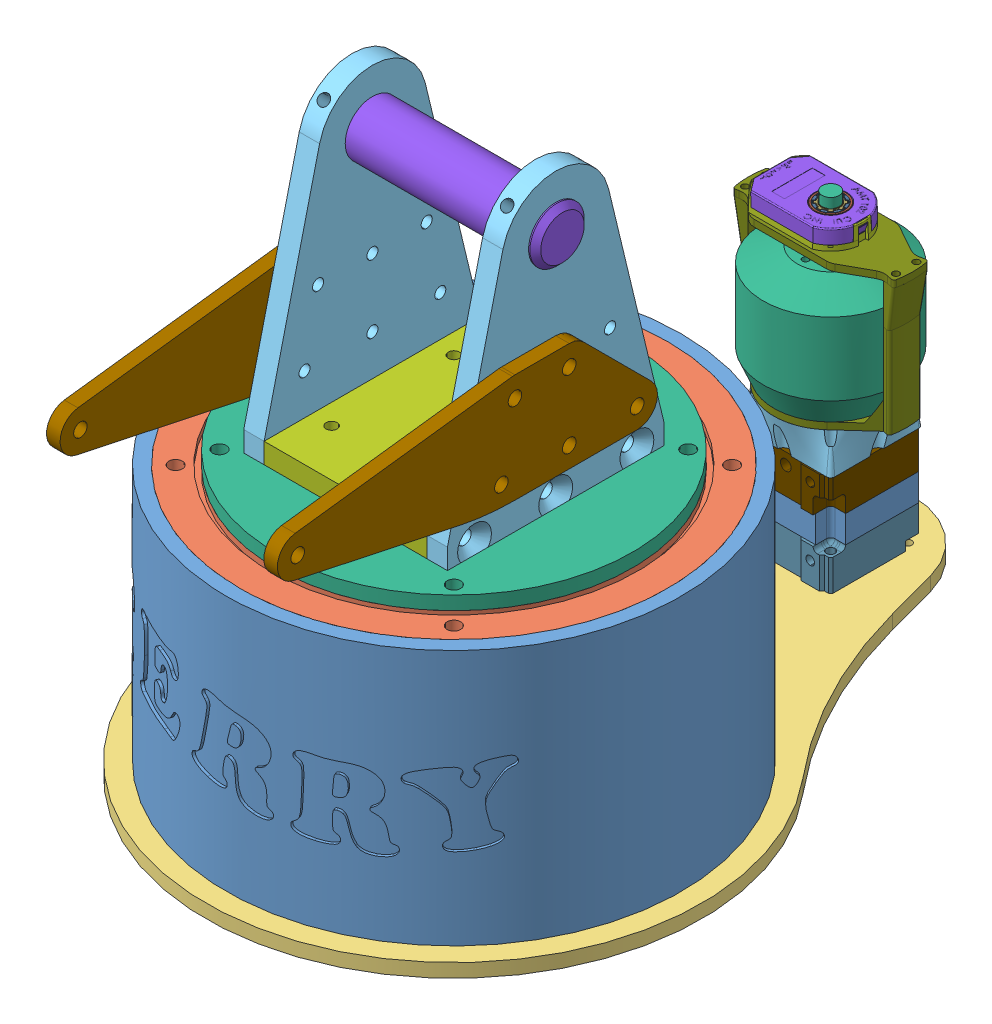
SolidWorks assembly Base, configuration Default. Lengths in mm.
Overall size (231.75 300.27 350.82).
75 component instances, 49 part files, 14 mates.
Components (placement in the parent):
- BotTurretHousing^Base-1: BotTurretHousing^Base [Default] at origin size (212.7 119.6 212.71) (virtual)
- 8in-1: 8in [Default] at (0 55.3 0) size (200 9 200)
- 8in-2: 8in [Default] at (0 -55.3 0) x (1 0 0) z (0 0 -1) size (200 9 200)
- BasePlate^Base-1: BasePlate^Base [Default] at origin size (231.75 6.35 330.18) (virtual)
- BotTurretPlate^Base-1: BotTurretPlate^Base [Default] at origin size (166.96 6.35 166.96) (virtual)
- SideTurretPlate^Base-1: SideTurretPlate^Base [Default] at origin size (9.52 262.48 101.23) (virtual)
- SideTurretPlate^Base-3: SideTurretPlate^Base [Default] x (-1 0 0) z (0 0 -1) size (9.52 262.48 101.23) (virtual)
- TopTurretPlate^Base-1: TopTurretPlate^Base [Default] at origin size (166.96 6.35 166.96) (virtual)
- TopBrace^Base-1: TopBrace^Base [Default] at origin size (76.2 9.53 101.23) (virtual)
- 6061K602_HARDENED PRECISION STEEL SHAFT-1: 6061K602_HARDENED PRECISION STEEL SHAFT [6061K602] at (0 177.275 0) size (101.6 25.4 25.4)
- PivotPlate^Base-1: PivotPlate^Base [Default] at origin size (6.35 50.8 177.8) (virtual)
- PivotPlate^Base-2: PivotPlate^Base [Default] at (101.6 0 0) size (6.35 50.8 177.8) (virtual)
- Keda9to1-1: Keda9to1 [Default] at (0 -43.175 -153.975) x (0 -1 0) z (1 0 0) size (176.96 63 76.93)
  - VersaPlanetary_v2_Single_Stage_10_1_with_BAG.STEP-1: VersaPlanetary_v2_Single_Stage_10_1_with_BAG.STEP [Default] at origin size (163.4 63.52 63.52)
    - 217-2820 Rev1_Public.STEP-1: 217-2820 Rev1_Public.STEP [Default] at (-4.6546 22.225 0) x (0 -0.456494 0.889726) z (-1 0 0) size (39.22 38.88 17.4)
      - 217-2625-100.STEP-1: 217-2625-100.STEP [Default] at origin size (39.22 38.88 12.7)
        - 217-2625-008 Rev1.STEP-1: 217-2625-008 Rev1.STEP [Default] at origin size (34.7 34.7 4.7)
        - 217-2625-010 Rev1.STEP-1: 217-2625-010 Rev1.STEP [Default] at (0 10.193 3.65) x (0.999813 0.019336 0) z (0 0 1) size (4 4 12)
        - 217-2625-010 Rev1.STEP-2: 217-2625-010 Rev1.STEP [Default] at (8.691 -5.3258 3.65) size (4 4 12)
        - 217-2625-010 Rev1.STEP-3: 217-2625-010 Rev1.STEP [Default] at (-8.691 -5.3258 3.65) size (4 4 12)
        - 217-2625-005 Rev1_Planet_Revolving_Follower01.STEP-1: 217-2625-005 Rev1_Planet_Revolving_Follower01.STEP [Default] at (8.691 -5.3258 6.35) x (0.932816 0.360354 0) z (0 0 1) size (16.89 16.89 8)
        - 217-2625-005 Rev1_Planet_Revolving_Follower01.STEP-2: 217-2625-005 Rev1_Planet_Revolving_Follower01.STEP [Default] at (-8.691 -5.3258 6.35) x (-0.932788 -0.360426 0) z (0 0 1) size (16.89 16.89 8)
        - 217-2625-005 Rev1_Planet_Revolving_Follower01.STEP-3: 217-2625-005 Rev1_Planet_Revolving_Follower01.STEP [Default] at (0 10.193 6.35) x (0.893583 0.448898 0) z (0 0 1) size (16.89 16.89 8)
      - 217-2625-007 Rev1_Public.STEP-1: 217-2625-007 Rev1_Public.STEP [Default] at (0 0 6.7) x (0.992772 0.120019 0) z (0 0 1) size (15.27 15.27 12.7)
    - 217-2625-026 Rev1.STEP-1: 217-2625-026 Rev1.STEP [Default] at (-6.5 22.225 0) x (0 -1 0) z (-1 0 0) size (44.45 42 18.12)
    - 217-2742-001 Rev4.STEP-1: 217-2742-001 Rev4.STEP [Default] at (0.2002 22.225 0) x (1 0 0) z (0 -0.092627 0.995701) size (7 28 28)
    - 217-2742-001 Rev4.STEP-2: 217-2742-001 Rev4.STEP [Default] at (8.2002 22.225 0) size (7 28 28)
    - 217-2625-017 Rev1_9714K61.STEP-1: 217-2625-017 Rev1_9714K61.STEP [Default] at (7.42 22.3002 -0.342) x (0 0.56703 0.823697) z (0 -0.823697 0.56703) size (28.51 4.98 27.43)
    - 217-2625-003 Rev1.STEP-1: 217-2625-003 Rev1.STEP [Default] at (7.4478 22.225 0) x (0 -1 0) z (1 0 0) size (17 17 64.11) (hidden)
    - 217-2625-018 Rev1_98541A410.STEP-1: 217-2625-018 Rev1_98541A410.STEP [Default] at (-0.7046 22.225 0) x (1 0 0) z (0 -0.017452 0.999848) size (1 19.6 17.4)
    - 832-1750-Ring-Gear-Screw_SSA0832-0500ZC.STEP-1: 832-1750-Ring-Gear-Screw_SSA0832-0500ZC.STEP [Default] at (-30.7 4.725 -17.5) x (0 0.997447 0.071411) z (0 -0.071411 0.997447) size (6.73 48.51 6.73) (hidden)
    - 832-1750-Ring-Gear-Screw_SSA0832-0500ZC.STEP-2: 832-1750-Ring-Gear-Screw_SSA0832-0500ZC.STEP [Default] at (-30.7 39.725 17.5) x (0 0.005929 0.999982) z (0 -0.999982 0.005929) size (6.73 48.51 6.73) (hidden)
    - 217-2625-025 Rev1.STEP-1: 217-2625-025 Rev1.STEP [Default] at (-23.2 22.225 0) x (0 -1 0) z (-1 0 0) size (44.45 42 18)
    - 217-4649-002 Rev1_SSA0832-0500ZC.STEP-1: 217-4649-002 Rev1_SSA0832-0500ZC.STEP [Default] at (-33.7 4.2645 17.9605) x (0 0.33842 -0.940995) z (0 0.940995 0.33842) size (6.73 16.76 6.73) (hidden)
    - 217-4649-002 Rev1_SSA0832-0500ZC.STEP-2: 217-4649-002 Rev1_SSA0832-0500ZC.STEP [Default] at (-33.7 40.1855 -17.9605) x (0 -0.308932 -0.951084) z (0 0.951084 -0.308932) size (6.73 16.76 6.73) (hidden)
    - 217-4649-006 Rev1_SSA0004-008BA.STEP-1: 217-4649-006 Rev1_SSA0004-008BA.STEP [Default] at (-30.7 22.225 12.5) x (0 0.5 -0.866025) z (0 -0.866025 -0.5) size (7 14 7) (hidden)
    - 217-4649-006 Rev1_SSA0004-008BA.STEP-2: 217-4649-006 Rev1_SSA0004-008BA.STEP [Default] at (-30.7 22.225 -12.5) x (0 -0.5 0.866025) z (0 0.866025 0.5) size (7 14 7) (hidden)
    - 217-2822-003 Rev4.STEP-1: 217-2822-003 Rev4.STEP [Default] at (-32.2 22.225 0) x (0 -1 0) z (-1 0 0) size (42 42 4.8) (hidden)
    - 217-3351 Rev2.STEP-1: 217-3351 Rev2.STEP [Default] at (-33.7 22.225 0) x (0 0 1) z (1 0 0) size (59.07 59.07 84.5) (hidden)
    - 217-2816-001 Rev1.STEP-1: 217-2816-001 Rev1.STEP [Default] at (-6.35 22.225 0) x (0 -1 0) z (1 0 0) size (42 42 14.51)
    - 217-4649-001 Rev1.STEP-1: 217-4649-001 Rev1.STEP [Default] at (-20.046 22.225 0) x (0 -1 0) z (1 0 0) size (18 18 13)
    - 217-4649-007 Rev1_94105A824.STEP-1: 217-4649-007 Rev1_94105A824.STEP [Default] at (-25.521 22.225 -6.7835) x (-0.996104 -0.088191 0) z (0 0 -1) size (4.83 4.83 4.77)
    - 217-2625-011 Rev1.STEP-1: 217-2625-011 Rev1.STEP [Default] at (-24.7818 22.225 0) x (0 0 1) z (0 -1 0) size (8.01 7.5 7.94) (hidden)
  - VersaPlanetary_CIM_Motor_Output_Shaft_Kit_217-2893-1: VersaPlanetary_CIM_Motor_Output_Shaft_Kit_217-2893 [Default] at (7.4478 22.225 0) x (0 0 -1) z (1 0 0) size (17 17 57.85)
  - KedaAdapter^Keda9to1-1: KedaAdapter^Keda9to1 [Default] at origin size (17.82 53.01 53.01) (virtual)
  - 192kvMotorEncoded-1: 192kvMotorEncoded [Default] at (-51.0318 22.225 0) x (0 -1 0) z (0 0 -1) size (63 104.52 76.93)
    - BetterKEDA-1: BetterKEDA [Default] at origin size (63 104.52 63)
    - CUI_DEVICES_AMT102-0048-N2000-S-1: CUI_DEVICES_AMT102-0048-N2000-S [Default] at (0 65.12 0) x (1 0 0) z (0 1 0) size (36.33 46.21 9.2)
      - CUI_DEVICES_AMT102-0048-N2000-S.step-1: CUI_DEVICES_AMT102-0048-N2000-S.step [Default] at origin size (36.33 46.21 9.2)
        - AMT-102-Base-REV-K.step-1: AMT-102-Base-REV-K.step [Default] x (-1 0 0) z (0 0 -1) size (28.78 43.39 9.06)
        - AMT-102-Top-Cover-REV-H.step-1: AMT-102-Top-Cover-REV-H.step [Default] at (0 0 5.23) x (-1 0 0) z (0 0 -1) size (28.6 43.26 6.55)
        - AMT-Sleeve-REV-D_ 2 mm.step-1: AMT-Sleeve-REV-D_ 2 mm.step [Default] at (0 0 -2.42) x (0.999996 0.002864 0) z (0 0 1) size (10.79 10.79 7.8)
        - AMT-Hub-Top-REV-D1.step-1: AMT-Hub-Top-REV-D1.step [Default] at (0 0 2.13) x (0.999996 0.002864 0) z (0 0 1) size (14 14 5.67)
        - AMT-Hub-Bottom-REV-B.step-1: AMT-Hub-Bottom-REV-B.step [Default] at (0 0 2.43) x (0.999998 -0.001942 0) z (0 0 1) size (17.3 17.3 3.2)
        - AMT10X-Shaft-Adaptor-REV-E.step-1: AMT10X-Shaft-Adaptor-REV-E.step [Default] at (0 0 0.03) x (0.999996 0.002864 0) z (0 0 1) size (11.8 11.8 7.8)
        - Receiver-board.step-1: Receiver-board.step [Default] at (72.2834 -20.351 3.03) x (-1 0 0) z (0 0 -1) size (26.5 26.62 0.41)
        - Rotor-board-REV F.step-1: Rotor-board-REV F.step [Default] at (0 0 2.13) x (0.807874 -0.589355 0) z (0 0 1) size (26 26 0.3)
        - Transmitter-board AMT10_AMT-102.step-1: Transmitter-board AMT10_AMT-102.step [Default] at (19.1596 -17.1102 1.22) x (-1 0 0) z (0 0 -1) size (26.63 38.43 4.41)
    - Body^192kvMotorEncoded-1: Body^192kvMotorEncoded [Default] at origin size (53 64.53 76.93) (virtual)
- J1Pulley-1: J1Pulley [Default] at (0 -92.675 0) size (144.68 26.53 144.68)
- 15Tpulley-2: 15Tpulley [Default] at (0 -84.675 -176.2) size (28 28 28)
- J1Belt^Base-1: J1Belt^Base [Default] at origin size (148.21 15.01 263.1) (virtual)
- TensionPillarJ1-1: TensionPillarJ1 [Default] at (-1.2541 -1.54 -8.5995) size (22.22 25.73 22.23)
  - 92510A774_ALUM UNTHRD SPACER-1-1: 92510A774_ALUM UNTHRD SPACER-1 [92510A774] at (20.3041 -69.3725 -110.4505) x (1 0 0) z (0 1 0) size (15.88 15.88 9.53)
  - 98019A228_MIL SPEC. 300 SERIES SS FLAT WASHER-1: 98019A228_MIL SPEC. 300 SERIES SS FLAT WASHER [98019A228] at (20.3041 -74.8462 -110.4505) x (0.972939 0 -0.231063) z (0.231063 0 0.972939) size (9.53 0.71 9.53)
  - 60355K701_BALL BEARING-1: 60355K701_BALL BEARING [60355K701] at (20.3041 -77.3354 -110.4505) x (1 0 0) z (0 1 0) size (15.88 15.88 4.98)
  - Roller^TensionPillarJ1-1: Roller^TensionPillarJ1 [Default] at (-2.0675 -17.1652 2.6827) size (22.23 15 22.23) (virtual)
  - 60355K701_BALL BEARING-2: 60355K701_BALL BEARING [60355K701] at (20.3041 -87.8548 -110.4505) x (1 0 0) z (0 1 0) size (15.88 15.88 4.98)
- TensionPillarJ1-2: TensionPillarJ1 [Default] at (1.2541 -1.54 -229.5005) x (-1 0 0) z (0 0 -1) size (22.22 25.73 22.23)
  - 92510A774_ALUM UNTHRD SPACER-1-1: 92510A774_ALUM UNTHRD SPACER-1 [92510A774] at (20.3041 -69.3725 -110.4505) x (1 0 0) z (0 1 0) size (15.88 15.88 9.53)
  - 98019A228_MIL SPEC. 300 SERIES SS FLAT WASHER-1: 98019A228_MIL SPEC. 300 SERIES SS FLAT WASHER [98019A228] at (20.3041 -74.8462 -110.4505) x (0.972939 0 -0.231063) z (0.231063 0 0.972939) size (9.53 0.71 9.53)
  - 60355K701_BALL BEARING-1: 60355K701_BALL BEARING [60355K701] at (20.3041 -77.3354 -110.4505) x (1 0 0) z (0 1 0) size (15.88 15.88 4.98)
  - Roller^TensionPillarJ1-1: Roller^TensionPillarJ1 [Default] at (-2.0675 -17.1652 2.6827) size (22.23 15 22.23) (virtual)
  - 60355K701_BALL BEARING-2: 60355K701_BALL BEARING [60355K701] at (20.3041 -87.8548 -110.4505) x (1 0 0) z (0 1 0) size (15.88 15.88 4.98)
- TensionConnector^Base-1: TensionConnector^Base [Default] at origin size (53.98 5.71 15.88) (virtual)
Mates (geometry in assembly coordinates):
- Concentric1: concentric aligned: cylinder of BotTurretHousing^Base-1 through (0 50.8 0) axis (0 -1 0) radius 86.02; cylinder of 8in-1 through (0 59.8 0) axis (0 -1 0) radius 69.5
- Coincident1: coincident anti-aligned: plane of BotTurretHousing^Base-1 through (0 50.8 0) normal (0 1 0); plane of 8in-1 through (0 50.8 0) normal (0 -1 0)
- Concentric3: concentric aligned: cylinder of SideTurretPlate^Base-2 through (38.1 177.275 0) axis (1 0 0) radius 12.7; cylinder of 6061K602_HARDENED PRECISION STEEL SHAFT-1 through (-50.8 177.275 0) axis (1 0 0) radius 12.7
- Width1: width anti-aligned: plane of 6061K602_HARDENED PRECISION STEEL SHAFT-1 through (50.8 177.275 0) normal (1 0 0); plane of SideTurretPlate^Base-1 through (-50.8 177.275 0) normal (-1 0 0); plane of 6061K602_HARDENED PRECISION STEEL SHAFT-1 through (-47.625 177.275 0) normal (-1 0 0); plane of SideTurretPlate^Base-3 through (47.625 177.275 0) normal (1 0 0)
- Concentric4: concentric anti-aligned: cylinder of BasePlate^Base-1 through (0 -66.15 -176.2) axis (0 1 0) radius 10; cylinder of Keda9to1-1/VersaPlanetary_CIM_Motor_Output_Shaft_Kit_217-2893-1 through (0 -58.3752 -176.2) axis (0 -1 0) radius 8.5
- Concentric5: concentric aligned: cylinder of BasePlate^Base-1 through (17.9605 -66.15 -158.2395) axis (0 1 0) radius 1.9844; cylinder of Keda9to1-1/VersaPlanetary_v2_Single_Stage_10_1_with_BAG.STEP-1/217-2625-026 Rev1.STEP-1 through (17.9605 -43.175 -158.2395) axis (0 1 0) radius 2.0193
- Coincident2: coincident anti-aligned: plane of BasePlate^Base-1 through (0 -59.8 0) normal (0 1 0); plane of Keda9to1-1/VersaPlanetary_v2_Single_Stage_10_1_with_BAG.STEP-1/217-2625-026 Rev1.STEP-1 through (22.225 -59.8 -198.425) normal (0 -1 0)
- Coincident3: coincident aligned: plane of J1Pulley-1 through (0 -92.675 0) normal (0 0 1)
- Coincident4: coincident aligned: plane of J1Pulley-1 through (0 -92.675 0) normal (1 0 0)
- Coincident7: coincident anti-aligned: plane of BotTurretPlate^Base-1 through (0 -66.15 0) normal (0 -1 0); plane of J1Pulley-1 through (0 -66.15 0) normal (0 1 0)
- Concentric6: concentric anti-aligned: cylinder of Keda9to1-1/VersaPlanetary_CIM_Motor_Output_Shaft_Kit_217-2893-1 through (0 -136.9432 -176.2) axis (0 1 0) radius 3.975; cylinder of 15Tpulley-2 through (0 -76.675 -176.2) axis (0 -1 0) radius 4
- Coincident8: coincident anti-aligned: plane of J1Pulley-1 through (0 -92.675 0) normal (0 -1 0); plane of 15Tpulley-2 through (0 -92.675 -176.2) normal (0 1 0)
- Coincident13: coincident anti-aligned: plane of BasePlate^Base-1 through (0 -66.15 0) normal (0 -1 0); plane of TensionPillar^Base-1/92510A774_ALUM UNTHRD SPACER-1-1 through (19.05 -66.15 -119.05) normal (0 1 0)
- Concentric12: concentric anti-aligned: cylinder of BasePlate^Base-1 through (19.05 -66.15 -119.05) axis (0 1 0) radius 3.175; cylinder of TensionPillar^Base-1/92510A774_ALUM UNTHRD SPACER-1-1 through (19.05 -66.15 -119.05) axis (0 -1 0) radius 3.2004
